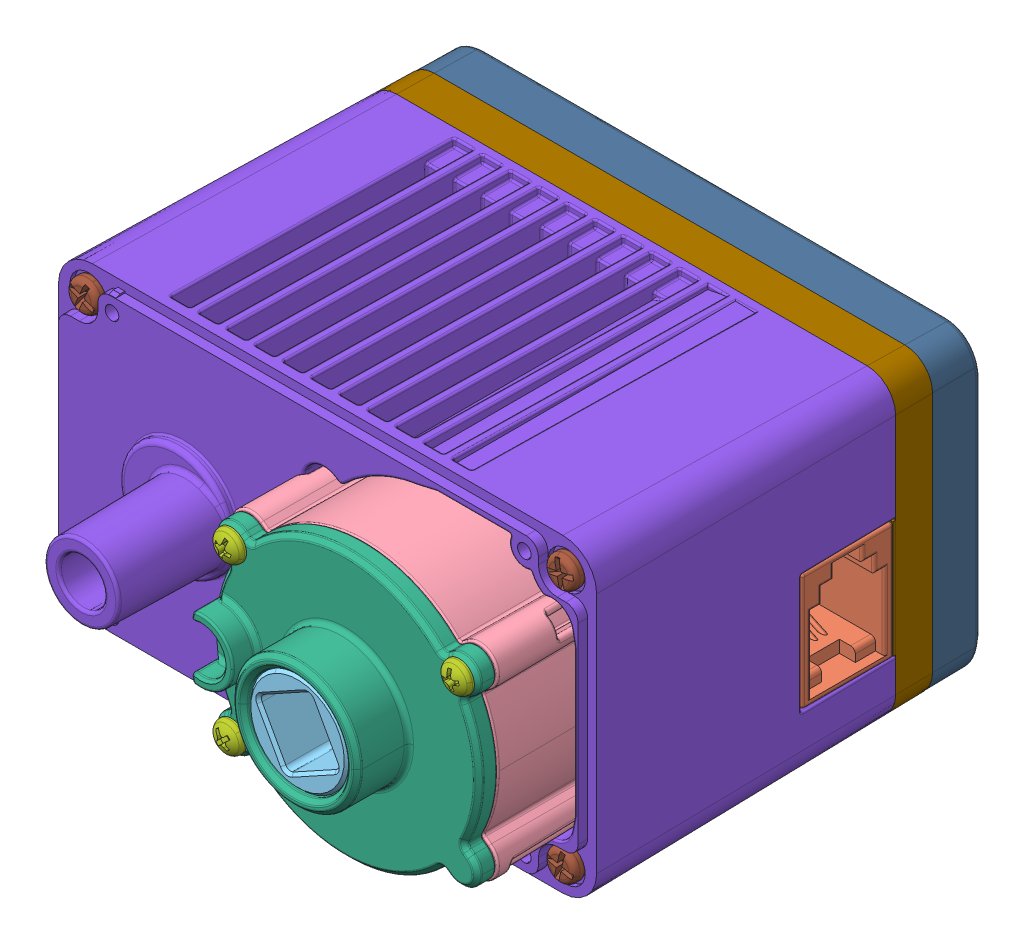
SolidWorks assembly V5 Smart Motor (276-4840).step, configuration Default. Lengths in mm.
Overall size (59.01 35.33 59.91).
19 component instances, 12 part files, 0 mates.
Components (placement in the parent):
- 276-4840-900 Rev6_Instruction.step-1: 276-4840-900 Rev6_Instruction.step [Default] at (-14.3 0 -17.2) size (52.79 15.94 38.15)
  - 276-4840-901 Rev6.step-1: 276-4840-901 Rev6.step [Default] at (10.75 -10.05 17.8) x (-1 0 0) z (0 0 1) size (49.9 1.6 38.15)
  - 276-4840-902 Rev2.step-1: 276-4840-902 Rev2.step [Default] at (31.25 -9.25 6.2) x (0 0 -1) z (0 -1 0) size (10.35 11.39 15.94)
  - 276-4840-022 Rev4.step-1: 276-4840-022 Rev4.step [Default] at (31.25 -9.25 6.2) x (0 0 -1) z (1 0 0) size (10.26 9.1 5.51)
- 276-4840-110 Rev10_Instruction.step-1: 276-4840-110 Rev10_Instruction.step [Default] at (12.7 0 14.7) size (35.33 35.33 31.1)
  - 276-4840-061 Rev7_Ring_Gear_Fixed01 .6 Rev3.step-1: 276-4840-061 Rev7_Ring_Gear_Fixed01 .6 Rev3.step [Default] at origin size (28.79 28.39 24.6)
  - 276-4840-018 Rev6.step-1: 276-4840-018 Rev6.step [Default] at (0 0 6.7) x (-0.483174 0.875524 0) z (0 0 1) size (26 26 12.3)
  - 276-4840-059 Rev2.step-1: 276-4840-059 Rev2.step [Default] at (0 0 10.3) size (28.4 28.4 8.5)
  - 276-4840-062 Rev1.step-1: 276-4840-062 Rev1.step [Default] at (-12.1353 8.8168 12.3) x (0.956835 -0.290632 0) z (-0.290632 -0.956835 0) size (3.2 6.56 3.2)
  - 276-4840-062 Rev1.step-2: 276-4840-062 Rev1.step [Default] at (12.1353 8.8168 12.3) x (0.978427 0.206591 0) z (0.206591 -0.978427 0) size (3.2 6.56 3.2)
  - 276-4840-062 Rev1.step-3: 276-4840-062 Rev1.step [Default] at (-12.1353 -8.8168 12.3) x (0.72563 0.688086 0) z (0.688086 -0.72563 0) size (3.2 6.56 3.2)
- 276-4840-001 Rev38.step-1: 276-4840-001 Rev38.step [Default] at origin size (57.3 33 46.9)
- 276-4840-005 Rev27.step-1: 276-4840-005 Rev27.step [Default] at (0 0 -17.95) size (56.17 31.87 12.9)
- 276-4840-004 Rev16.step-1: 276-4840-004 Rev16.step [Default] at (0 0 -19.2) size (56.01 31.71 9.21)
- 276-4840-009 Rev3.step-1: 276-4840-009 Rev3.step [Default] at (25.45 13.5 15.7) x (0.19987 -0.979823 0) z (-0.979823 -0.19987 0) size (3.4 41.31 4.34)
- 276-4840-009 Rev3.step-2: 276-4840-009 Rev3.step [Default] at (-25.45 -13.5 15.7) x (-0.998855 0.047836 0) z (0.047836 0.998855 0) size (3.4 41.31 4.34)
- 276-4840-009 Rev3.step-3: 276-4840-009 Rev3.step [Default] at (25.45 -13.5 15.7) x (-0.975374 0.220559 0) z (0.220559 0.975374 0) size (3.4 41.31 4.34)
- 276-4840-009 Rev3.step-4: 276-4840-009 Rev3.step [Default] at (-25.45 13.5 15.7) x (-0.922256 0.38658 0) z (0.38658 0.922256 0) size (3.4 41.31 4.34)
- 276-4840-025 Rev19.step-1: 276-4840-025 Rev19.step [Default] at (12.7 0 -22.63) x (-0.993315 0.115437 0) z (0 0 1) size (14.82 14.83 35.18)
